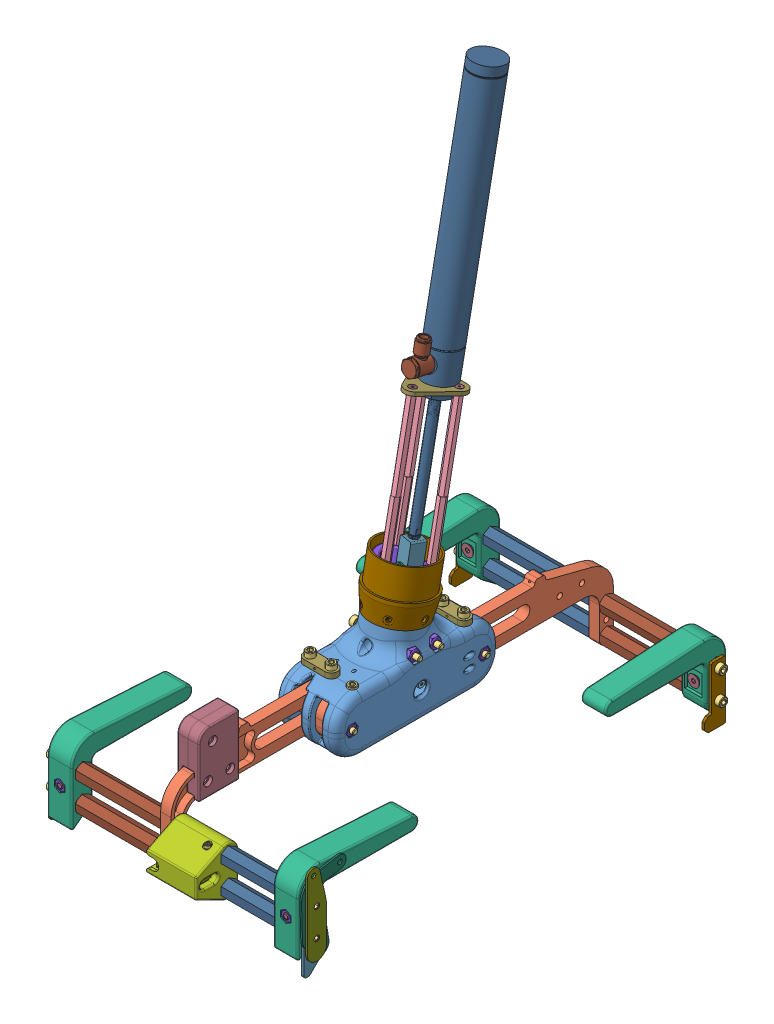
SolidWorks assembly 971-18-A-4000_The Claw, configuration Default. Lengths in mm.
Overall size (243.27 530.53 410.02).
118 component instances, 34 part files, 272 mates.
Components (placement in the parent):
- 971-18-P-0108_Printed Claw Body-1: 971-18-P-0108_Printed Claw Body [Default] at origin size (58.05 92.05 149.22)
- 971-18-P-0077_Main Claw plate-2: 971-18-P-0077_Main Claw plate [Main Claw plate revised] at (9.4298 -158.75 -26.9875) x (0 0 1) z (-1 0 0) size (261.94 82.88 9.53)
- 971-18-P-0077_Main Claw plate-3: 971-18-P-0077_Main Claw plate [Main Claw plate revised] at (-9.4298 -158.75 26.9875) x (0 0 -1) z (1 0 0) size (261.94 82.88 9.53)
- SHCS-1: SHCS [2.25, #10-32] at (3.175 0 -60.325) x (1 0 0) z (0 0.140282 0.990112) size (61.98 7.92 7.92)
- SHCS-2: SHCS [2.25, #10-32] at (3.175 0 60.325) x (1 0 0) z (0 0.980553 -0.196257) size (61.98 7.92 7.92)
- SHCS-3: SHCS [1.875, #10-32] at (-19.177 -1.5875 -50.8) x (0 -1 0) z (-0.074372 0 -0.997231) size (52.45 7.92 7.92)
- SHCS-8: SHCS [2.25, #10-32] at (0 1.5875 -50.8) x (0 -1 0) z (-0.997477 0 -0.07099) size (61.98 7.92 7.92)
- SHCS-9: SHCS [2.25, #10-32] at (19.177 1.5875 -50.8) x (0 -1 0) z (-0.818231 0 -0.57489) size (61.98 7.92 7.92)
- SHCS-10: SHCS [1.875, #10-32] at (19.177 -1.5875 50.8) x (0 -1 0) z (-0.72422 0 -0.689569) size (52.45 7.92 7.92)
- SHCS-11: SHCS [2.25, #10-32] at (0 1.5875 50.8) x (0 -1 0) z (-0.999175 0 0.040609) size (61.98 7.92 7.92)
- SHCS-12: SHCS [2.25, #10-32] at (-19.177 1.5875 50.8) x (0 -1 0) z (0.998979 0 0.045167) size (61.98 7.92 7.92)
- 9433K640_PRECISION STAINLESS STEEL EXTENSION SPRING-1: 9433K640_PRECISION STAINLESS STEEL EXTENSION SPRING [9433K64] at (18.9548 0 -18.9695) x (0 0 1) z (-1 0 0) size (39.67 9.89 9.66)
- 91259A155_ALLOY STEEL SHOULDER SCREW-1: 91259A155_ALLOY STEEL SHOULDER SCREW [91259A155] at (20.5423 0 -7.9375) x (0 -0.354679 -0.934988) z (0 -0.934988 0.354679) size (6.35 13.86 6.35)
- 91259A155_ALLOY STEEL SHOULDER SCREW-2: 91259A155_ALLOY STEEL SHOULDER SCREW [91259A155] at (-20.5423 0 -34.9538) x (0 -0.751431 0.659812) z (0 -0.659812 -0.751431) size (6.35 13.86 6.35)
- 9433K640_PRECISION STAINLESS STEEL EXTENSION SPRING-2: 9433K640_PRECISION STAINLESS STEEL EXTENSION SPRING [9433K64] at (-18.9548 0 20.6375) x (0 0 1) z (-1 0 0) size (39.67 9.89 9.66)
- Bearings-1: Bearings [0.1875 ID, 0.375 OD, 0.125 Width, R166-2Z] at (9.3662 27.94 -18.3873) x (0 -0.996654 0.08174) z (1 0 0) size (9.53 9.53 3.17)
- Bearings-2: Bearings [0.1875 ID, 0.375 OD, 0.125 Width, R166-2Z] at (-9.4932 27.94 1.0215) x (0 -0.380852 0.924636) z (1 0 0) size (9.53 9.53 3.17)
- 971-18-P-0120_Printed Claw Pulley-3: 971-18-P-0120_Printed Claw Pulley [Default] at (-9.4298 27.94 1.0215) x (0 0.87562 0.483001) z (-1 0 0) size (19.05 19.05 4.76)
- 971-18-P-0120_Printed Claw Pulley-4: 971-18-P-0120_Printed Claw Pulley [Default] at (9.4298 27.94 -18.3873) x (0 -0.06152 0.998106) z (-1 0 0) size (19.05 19.05 4.76)
- SHCS-13: SHCS [2.25, #10-32] at (3.175 27.94 -18.3873) x (1 0 0) z (0 0.140282 0.990112) size (61.98 7.92 7.92)
- SHCS-14: SHCS [2.25, #10-32] at (3.175 27.94 1.0215) x (1 0 0) z (0 0.140282 0.990112) size (61.98 7.92 7.92)
- Nylon-Insert Locknut-1: Nylon-Insert Locknut [#10-32 Thin Nylon-Insert Locknut] at (22.225 27.94 1.0215) x (0 -0.5 -0.866025) z (0 -0.866025 0.5) size (9.53 4.37 11)
- Nylon-Insert Locknut-2: Nylon-Insert Locknut [#10-32 Thin Nylon-Insert Locknut] at (22.225 27.94 -18.3873) x (0 1 0) z (0 0 -1) size (9.53 4.37 11)
- Nylon-Insert Locknut-4: Nylon-Insert Locknut [#10-32 Thin Nylon-Insert Locknut] at (24.2094 0 -60.325) x (0 -0.5 -0.866025) z (0 -0.866025 0.5) size (9.53 4.37 11)
- Nylon-Insert Locknut-5: Nylon-Insert Locknut [#10-32 Thin Nylon-Insert Locknut] at (24.2094 0 60.325) x (0 -0.5 0.866025) z (0 0.866025 0.5) size (9.53 4.37 11)
- Nylon-Insert Locknut-14: Nylon-Insert Locknut [#10-32 Thin Nylon-Insert Locknut] at (19.177 -21.0344 50.8) x (0.5 0 0.866025) z (0.866025 0 -0.5) size (9.53 4.37 11)
- Nylon-Insert Locknut-15: Nylon-Insert Locknut [#10-32 Thin Nylon-Insert Locknut] at (0 -21.0344 50.8) x (-0.5 0 -0.866025) z (-0.866025 0 0.5) size (9.53 4.37 11)
- Nylon-Insert Locknut-17: Nylon-Insert Locknut [#10-32 Thin Nylon-Insert Locknut] at (-19.177 -21.0344 50.8) x (-0.5 0 -0.866025) z (-0.866025 0 0.5) size (9.53 4.37 11)
- Nylon-Insert Locknut-18: Nylon-Insert Locknut [#10-32 Thin Nylon-Insert Locknut] at (0 -21.0344 -50.8) x (1 0 0) z (0 0 -1) size (9.53 4.37 11)
- Nylon-Insert Locknut-19: Nylon-Insert Locknut [#10-32 Thin Nylon-Insert Locknut] at (-19.177 -21.0344 -50.8) x (0.5 0 -0.866025) z (-0.866025 0 -0.5) size (9.53 4.37 11)
- Nylon-Insert Locknut-20: Nylon-Insert Locknut [#10-32 Thin Nylon-Insert Locknut] at (19.177 -21.0344 -50.8) x (-0.5 0 0.866025) z (0.866025 0 0.5) size (9.53 4.37 11)
- 971-18-P-0142_Distal Carbon tube adapter-1: 971-18-P-0142_Distal Carbon tube adapter [Default] at (0 89.7497 -17.5007) x (-0.5 -0.165748 -0.850016) z (0 0.981514 -0.19139) size (53.98 53.98 46.99)
- 6498K084_ROUND BODY AIR CYLINDER-1: 6498K084_ROUND BODY AIR CYLINDER [6498K084] at (0 262.1497 -57.0582) x (0 0.981514 -0.19139) z (0 0.19139 0.981514) size (365.16 28.45 28.45)
- 5779K652_PUSH-TO-CONNECT TUBE FITTING FOR AIR-1: 5779K652_PUSH-TO-CONNECT TUBE FITTING FOR AIR [5779K652] at (0 225.7462 -44.6778) x (-1 0 0) z (0 -0.19139 -0.981514) size (14.22 28.59 25.52)
- 971-18-P-0153_Claw Piston Mount-1: 971-18-P-0153_Claw Piston Mount [Default] at (0 207.2186 -46.3469) x (-1 0 0) z (0 -0.19139 -0.981514) size (45.75 3.17 41.53)
- FHCS-15: FHCS [0.25, #4-40] at (-15.7499 209.7238 -50.0883) x (-0.913608 0.077818 0.39908) z (0 0.981514 -0.19139) size (6.48 6.48 6.43)
- FHCS-18: FHCS [0.25, #4-40] at (15.7499 209.7238 -50.0883) x (-0.453098 0.170616 0.874981) z (0 0.981514 -0.19139) size (6.48 6.48 6.43)
- FHCS-17: FHCS [0.25, #4-40] at (0 214.9449 -23.313) x (-0.453098 0.170616 0.874981) z (0 0.981514 -0.19139) size (6.48 6.48 6.43)
- 971-18-P-0162_Claw Piston Cable Block-1: 971-18-P-0162_Claw Piston Cable Block [Default] at (0 80.0327 -21.5464) x (0.973108 0.044086 0.22609) z (-0.230348 0.186243 0.95512) size (12.7 31.75 12.7)
- SHCS-19: SHCS [0.875, #10-32] at (0.7167 71.3508 -22.9383) x (0.230348 -0.186243 -0.95512) z (0.455328 -0.84681 0.274935) size (27.05 7.92 7.92)
- Nylon-Insert Locknut-21: Nylon-Insert Locknut [#10-32 Thin Nylon-Insert Locknut] at (1.843 70.4402 -27.6084) x (-0.550845 -0.834076 0.029792) z (0.802191 -0.51926 0.294719) size (9.53 4.37 11)
- SAE Washer, 18-8 Stainless Steel-1: SAE Washer, 18-8 Stainless Steel [No. 10 Screw SAE Washer] at (-1.6529 73.2667 -13.113) x (0.166548 0.974577 -0.14987) z (0.95875 -0.124551 0.25551) size (12.7 1.65 12.7)
- SAE Washer, 18-8 Stainless Steel-2: SAE Washer, 18-8 Stainless Steel [No. 10 Screw SAE Washer] at (1.6529 70.5939 -26.8199) x (0.166548 0.974577 -0.14987) z (0.95875 -0.124551 0.25551) size (12.7 1.65 12.7)
- FHCS-19: FHCS [0.25, #4-40] at (0 214.9449 -23.313) x (-0.309292 0.182005 0.933388) z (0 0.981514 -0.19139) size (6.48 6.48 6.43)
- Beam Diffuse Sensor-1: Beam Diffuse Sensor [Default] at (2.3678 -35.946 191.135) x (0 -1 0) z (0 0 1) size (12.7 33.5 22.88)
- SHCS-24: SHCS [1, #10-32] at (-103.6637 -29.5056 185.7375) x (1 0 0) z (0 0.235318 -0.971918) size (30.45 7.92 7.92)
- SHCS-26: SHCS [1.5, #4-40] at (30.5617 -43.439 194.183) x (0 -1 0) z (0.977714 0 0.209939) size (40.94 4.65 4.65)
- SHCS-33: SHCS [1, #10-32] at (103.6637 -29.5056 185.7375) x (-1 0 0) z (0 0.845438 -0.534073) size (30.45 7.92 7.92)
- SHCS-35: SHCS [1, #10-32] at (103.6637 -54.9056 185.7375) x (-1 0 0) z (0 -0.631694 -0.775218) size (30.45 7.92 7.92)
- SHCS-37: SHCS [1, #10-32] at (103.6637 -29.5056 -185.7375) x (-1 0 0) z (0 -0.058563 -0.998284) size (30.45 7.92 7.92)
- SHCS-39: SHCS [1, #10-32] at (103.6637 -54.9056 -185.7375) x (-1 0 0) z (0 -0.744643 -0.667463) size (30.45 7.92 7.92)
- SHCS-41: SHCS [1, #10-32] at (-103.6637 -54.9056 -185.7375) x (1 0 0) z (0 0.359883 -0.932997) size (30.45 7.92 7.92)
- SHCS-43: SHCS [1, #10-32] at (-103.6637 -29.5056 -185.7375) x (1 0 0) z (0 0.980192 0.198051) size (30.45 7.92 7.92)
- 92311A433_18-8 SS CUP POINT SET SCREW-1: 92311A433_18-8 SS CUP POINT SET SCREW [92311A433] at (-10.0105 -54.9056 185.7375) x (0 -0.712759 -0.701409) z (-1 0 0) size (4.99 4.84 25.82)
- 92311A433_18-8 SS CUP POINT SET SCREW-5: 92311A433_18-8 SS CUP POINT SET SCREW [92311A433] at (-11.02 -29.5056 185.7375) x (0 -0.999929 0.011906) z (1 0 0) size (4.99 4.84 25.82)
- 93365A142_BRASS HEAT-SET INSERT FOR PLASTICS-1: 93365A142_BRASS HEAT-SET INSERT FOR PLASTICS [93365A142] at (-11.1125 53.5447 9.169) x (0.785545 0.5 0.36458) z (0.36458 -0.850016 0.380203) size (6.35 8.46 6.35)
- 93365A142_BRASS HEAT-SET INSERT FOR PLASTICS-2: 93365A142_BRASS HEAT-SET INSERT FOR PLASTICS [93365A142] at (-22.225 49.8609 -9.7226) x (0 0.545272 0.838259) z (0 -0.838259 0.545272) size (6.35 8.46 6.35)
- 93365A142_BRASS HEAT-SET INSERT FOR PLASTICS-4: 93365A142_BRASS HEAT-SET INSERT FOR PLASTICS [93365A142] at (-11.1125 46.1772 -28.6142) x (-0.813186 -0.24774 0.526644) z (0.297873 -0.954543 0.010914) size (6.35 8.46 6.35)
- 93365A142_BRASS HEAT-SET INSERT FOR PLASTICS-6: 93365A142_BRASS HEAT-SET INSERT FOR PLASTICS [93365A142] at (11.1125 46.1772 -28.6142) x (0.371763 0.927557 0.037811) z (-0.782172 0.33491 -0.525398) size (6.35 8.46 6.35)
- 93365A142_BRASS HEAT-SET INSERT FOR PLASTICS-8: 93365A142_BRASS HEAT-SET INSERT FOR PLASTICS [93365A142] at (22.225 49.8609 -9.7226) x (0 0.873561 -0.486714) z (0 -0.486714 -0.873561) size (6.35 8.46 6.35)
- 93365A142_BRASS HEAT-SET INSERT FOR PLASTICS-10: 93365A142_BRASS HEAT-SET INSERT FOR PLASTICS [93365A142] at (11.1125 53.5447 9.169) x (0.459987 0.780789 -0.422825) z (0.733766 -0.602409 -0.314152) size (6.35 8.46 6.35)
- 92311A433_18-8 SS CUP POINT SET SCREW-11: 92311A433_18-8 SS CUP POINT SET SCREW [92311A433] at (9.2914 -29.5056 -185.7375) x (0 0.990314 -0.138846) z (1 0 0) size (4.99 4.84 25.82)
- 92311A433_18-8 SS CUP POINT SET SCREW-14: 92311A433_18-8 SS CUP POINT SET SCREW [92311A433] at (9.9158 -54.9056 -185.7375) x (0 -0.994426 -0.105437) z (1 0 0) size (4.99 4.84 25.82)
- 94638A222_NYLON UNTHREADED SPACERS-1: 94638A222_NYLON UNTHREADED SPACERS [94638A222] at (-19.177 0 50.8) x (1 0 0) z (0 1 0) size (9.53 9.53 33.34)
- 94638A222_NYLON UNTHREADED SPACERS-2: 94638A222_NYLON UNTHREADED SPACERS [94638A222] at (-19.177 0 -50.8) x (1 0 0) z (0 1 0) size (9.53 9.53 33.34)
- 94638A222_NYLON UNTHREADED SPACERS-3: 94638A222_NYLON UNTHREADED SPACERS [94638A222] at (19.177 0 -50.8) x (1 0 0) z (0 1 0) size (9.53 9.53 33.34)
- 94639A550_NYLON UNTHREADED SPACERS-1: 94639A550_NYLON UNTHREADED SPACERS [94639A550] at (-9.4298 0 -60.325) x (0 -0.918334 -0.395806) z (1 0 0) size (12.7 12.7 9.53)
- 94639A586_NYLON UNTHREADED SPACERS-1: 94639A586_NYLON UNTHREADED SPACERS [94639A586] at (0 11.9062 50.8) x (1 0 0) z (0 1 0) size (9.53 9.53 10.32)
- 94638A222_NYLON UNTHREADED SPACERS-4: 94638A222_NYLON UNTHREADED SPACERS [94638A222] at (19.177 0 50.8) x (1 0 0) z (0 1 0) size (9.53 9.53 33.34)
- 94639A550_NYLON UNTHREADED SPACERS-2: 94639A550_NYLON UNTHREADED SPACERS [94639A550] at (9.4298 0 -60.325) x (0 -0.323653 0.946176) z (-1 0 0) size (12.7 12.7 9.53)
- 94639A550_NYLON UNTHREADED SPACERS-3: 94639A550_NYLON UNTHREADED SPACERS [94639A550] at (-9.4298 0 60.325) x (0 -0.362888 0.931833) z (-1 0 0) size (12.7 12.7 9.53)
- 94639A550_NYLON UNTHREADED SPACERS-4: 94639A550_NYLON UNTHREADED SPACERS [94639A550] at (9.4298 0 60.325) x (0 -0.966697 0.255924) z (-1 0 0) size (12.7 12.7 9.53)
- 94639A586_NYLON UNTHREADED SPACERS-2: 94639A586_NYLON UNTHREADED SPACERS [94639A586] at (0 11.9062 -50.8) x (1 0 0) z (0 1 0) size (9.53 9.53 10.32)
- 94639A586_NYLON UNTHREADED SPACERS-3: 94639A586_NYLON UNTHREADED SPACERS [94639A586] at (0 -11.9062 50.8) x (1 0 0) z (0 1 0) size (9.53 9.53 10.32)
- 94639A586_NYLON UNTHREADED SPACERS-4: 94639A586_NYLON UNTHREADED SPACERS [94639A586] at (0 -11.9062 -50.8) x (1 0 0) z (0 1 0) size (9.53 9.53 10.32)
- 91780A049_ALUM FEM THRDED HEX STANDOFF-1: 91780A049_ALUM FEM THRDED HEX STANDOFF [91780A049] at (0 174.4329 -15.4133) x (0.203683 0.187378 0.960938) z (0 -0.981514 0.19139) size (6.35 7.33 76.64)
- 98637A123_ALLOY STEEL MIL SPEC CUP POINT SET SCREW-1: 98637A123_ALLOY STEEL MIL SPEC CUP POINT SET SCREW [98637A123] at (0 134.5273 -7.632) x (0.994254 0.020488 0.105072) z (0 -0.981514 0.19139) size (3.28 2.93 13.1)
- SHCS-44: SHCS [1, #10-32] at (-103.6637 -54.9056 185.7375) x (1 0 0) z (0 0.985655 0.168775) size (30.45 7.92 7.92)
- 91780A049_ALUM FEM THRDED HEX STANDOFF-2: 91780A049_ALUM FEM THRDED HEX STANDOFF [91780A049] at (15.7499 94.4205 -27.6048) x (-0.911227 0.078834 0.404291) z (0 0.981514 -0.19139) size (6.35 7.33 76.64)
- 91780A049_ALUM FEM THRDED HEX STANDOFF-3: 91780A049_ALUM FEM THRDED HEX STANDOFF [91780A049] at (-15.7499 169.2118 -42.1887) x (1 0 0) z (0 0.981514 -0.19139) size (6.35 7.33 76.64)
- 91780A049_ALUM FEM THRDED HEX STANDOFF-4: 91780A049_ALUM FEM THRDED HEX STANDOFF [91780A049] at (-15.7499 94.4205 -27.6048) x (-0.005423 -0.191387 -0.9815) z (0 -0.981514 0.19139) size (6.35 7.33 76.64)
- 91780A049_ALUM FEM THRDED HEX STANDOFF-5: 91780A049_ALUM FEM THRDED HEX STANDOFF [91780A049] at (15.7499 169.2118 -42.1887) x (-0.577436 0.156258 0.801344) z (0 0.981514 -0.19139) size (6.35 7.33 76.64)
- 91780A049_ALUM FEM THRDED HEX STANDOFF-6: 91780A049_ALUM FEM THRDED HEX STANDOFF [91780A049] at (0 99.6415 -0.8294) x (0.866025 -0.095695 -0.490757) z (0 -0.981514 0.19139) size (6.35 7.33 76.64)
- 98637A123_ALLOY STEEL MIL SPEC CUP POINT SET SCREW-2: 98637A123_ALLOY STEEL MIL SPEC CUP POINT SET SCREW [98637A123] at (-15.7499 132.8293 -35.0943) x (-0.962053 0.052223 0.267819) z (0 0.981514 -0.19139) size (3.28 2.93 13.1)
- 98637A123_ALLOY STEEL MIL SPEC CUP POINT SET SCREW-3: 98637A123_ALLOY STEEL MIL SPEC CUP POINT SET SCREW [98637A123] at (15.7499 131.8727 -34.9077) x (-0.341225 -0.179903 -0.922605) z (0 -0.981514 0.19139) size (3.28 2.93 13.1)
- 971-18-P-0299_Printed Claw Ends-1: 971-18-P-0299_Printed Claw Ends [Default] at (102.9652 -29.5056 -185.7375) size (22.23 68.03 110.13)
- 971-18-P-0299_Printed Claw Ends-2: 971-18-P-0299_Printed Claw Ends [Default] at (-102.9652 -29.5056 -185.7375) size (22.23 68.03 110.13)
- 971-18-P-0299_Printed Claw Ends-3: 971-18-P-0299_Printed Claw Ends [Default] at (-102.9652 -29.5056 185.7375) x (-1 0 0) z (0 0 -1) size (22.23 68.03 110.13)
- 971-18-P-0299_Printed Claw Ends-4: 971-18-P-0299_Printed Claw Ends [Default] at (102.9652 -29.5056 185.7375) x (-1 0 0) z (0 0 -1) size (22.23 68.03 110.13)
- 971-18-P-0300_Printed Claw Beam Break Mount-1: 971-18-P-0300_Printed Claw Beam Break Mount [Default] at (18.1928 -29.469 185.801) x (-1 0 0) z (0 0 -1) size (45.72 44.45 38.48)
- Nylon-Insert Locknut-22: Nylon-Insert Locknut [#10-32 Thin Nylon-Insert Locknut] at (102.9652 -42.2056 190.5) x (-0.998457 -0.055527 0) z (-0.055527 0.998457 0) size (9.53 4.37 11)
- FHCS-20: FHCS [0.75, #10-32] at (102.9652 -42.2056 176.2125) x (-0.923728 -0.383049 0) z (0 0 -1) size (10.44 10.44 19.21)
- FHCS-21: FHCS [0.75, #10-32] at (-102.9652 -42.2056 176.2125) x (-0.873774 -0.486332 0) z (0 0 -1) size (10.44 10.44 19.21)
- FHCS-24: FHCS [0.75, #10-32] at (-102.9652 -42.2056 -176.2125) x (-0.044015 -0.999031 0) z (0 0 1) size (10.44 10.44 19.21)
- FHCS-26: FHCS [0.75, #10-32] at (102.9652 -42.2056 -176.2125) x (0.130134 -0.991496 0) z (0 0 1) size (10.44 10.44 19.21)
- Nylon-Insert Locknut-23: Nylon-Insert Locknut [#10-32 Thin Nylon-Insert Locknut] at (-102.9652 -42.2056 190.5) x (-0.985526 -0.169524 0) z (-0.169524 0.985526 0) size (9.53 4.37 11)
- Nylon-Insert Locknut-25: Nylon-Insert Locknut [#10-32 Thin Nylon-Insert Locknut] at (-102.9652 -42.2056 -190.5) x (0.289314 -0.957234 0) z (0.957234 0.289314 0) size (9.53 4.37 11)
- Nylon-Insert Locknut-27: Nylon-Insert Locknut [#10-32 Thin Nylon-Insert Locknut] at (102.9652 -42.2056 -190.5) x (0.451141 -0.892453 0) z (0.892453 0.451141 0) size (9.53 4.37 11)
- 971-18-P-0304_Claw Standoff Ring-1: 971-18-P-0304_Claw Standoff Ring [Default] at (0 65.555 -12.7829) x (0.5 0.165748 0.850016) z (-0.866025 0.095695 0.490757) size (43.02 19.34 44.45)
- 971-18-P-0312_Claw Fangs-1: 971-18-P-0312_Claw Fangs [Default] at (114.0778 -76.4956 200.7755) size (2.29 53.34 19.05) (hidden)
- 971-18-P-0312_Claw Fangs-6: 971-18-P-0312_Claw Fangs [Default] at (-114.0778 -76.4956 -200.7755) x (-1 0 0) z (0 0 -1) size (2.29 53.34 19.05)
- 971-18-P-0312_Claw Fangs-11: 971-18-P-0312_Claw Fangs [Default] at (116.3637 -76.4956 -200.7755) x (-1 0 0) z (0 0 -1) size (2.29 53.34 19.05)
- 971-18-P-0312_Claw Fangs-12: 971-18-P-0312_Claw Fangs [Default] at (-116.3637 -76.4956 200.7755) size (2.29 53.34 19.05)
- 971-18-P-0316_Claw Long Horizontal Standoff-1: 971-18-P-0316_Claw Long Horizontal Standoff [91780A354] at (-46.1328 -54.9056 -185.7375) x (0 0.866025 -0.5) z (1 0 0) size (12.7 14.66 102.22)
- 971-18-P-0317_Claw Short Horizontal Standoff-1: 971-18-P-0317_Claw Short Horizontal Standoff [91780A354] at (-91.8528 -54.9056 185.7375) x (0 -0.912023 0.41014) z (1 0 0) size (12.7 14.66 82.74)
- 971-18-P-0317_Claw Short Horizontal Standoff-2: 971-18-P-0317_Claw Short Horizontal Standoff [91780A354] at (91.8528 -54.9056 -185.7375) x (0 -0.866025 0.5) z (-1 0 0) size (12.7 14.66 82.74)
- 971-18-P-0317_Claw Short Horizontal Standoff-3: 971-18-P-0317_Claw Short Horizontal Standoff [91780A354] at (91.8528 -29.5056 -185.7375) x (0 0.196892 -0.980425) z (-1 0 0) size (12.7 14.66 82.74)
- 971-18-P-0317_Claw Short Horizontal Standoff-4: 971-18-P-0317_Claw Short Horizontal Standoff [91780A354] at (-91.8528 -29.5056 185.7375) x (0 0.866025 -0.5) z (1 0 0) size (12.7 14.66 82.74)
- 971-18-P-0316_Claw Long Horizontal Standoff-2: 971-18-P-0316_Claw Long Horizontal Standoff [91780A354] at (46.1328 -29.5056 185.7375) x (0 0 1) z (-1 0 0) size (12.7 14.66 102.22)
- 971-18-P-0316_Claw Long Horizontal Standoff-3: 971-18-P-0316_Claw Long Horizontal Standoff [91780A354] at (-46.1328 -29.5056 -185.7375) x (0 0.866025 -0.5) z (1 0 0) size (12.7 14.66 102.22)
- 971-18-P-0316_Claw Long Horizontal Standoff-4: 971-18-P-0316_Claw Long Horizontal Standoff [91780A354] at (46.1328 -54.9056 185.7375) x (0 0.866025 -0.5) z (-1 0 0) size (12.7 14.66 102.22)
- 971-18-P-0326_Claw Cable Holder-2: 971-18-P-0326_Claw Cable Holder [Default] at (-19.177 30.1625 50.8) x (1 0 0) z (0 0 -1) size (30.61 4.76 11.43)
- 971-18-P-0326_Claw Cable Holder-3: 971-18-P-0326_Claw Cable Holder [Default] at (0 30.1625 -50.8) x (1 0 0) z (0 0 -1) size (30.61 4.76 11.43)
- 971-18-P-0318_Claw Pulley Mount-5: 971-18-P-0318_Claw Pulley Mount [971-18-P-0318_Claw Pulley Mount] at (-19.2722 5.212 171.7608) x (0 0 -1) z (1 0 0) size (36.91 55.31 10.39)
- 971-18-P-0318_Claw Pulley Mount-6: 971-18-P-0318_Claw Pulley Mount [971-18-P-0330_Claw Pulley Mount Inner Side] at (-9.4298 5.212 171.7608) x (0 0 -1) z (1 0 0) size (36.91 55.31 11.43)
- 971-18-P-0361_Claw Fangs V2-1: 971-18-P-0361_Claw Fangs V2 [Default] at (115.2207 -29.5056 185.7375) size (2.29 63.5 20.32)
- 971-18-P-0367_Retrofit Fang Sheath-1: 971-18-P-0367_Retrofit Fang Sheath [Default] at (116.3637 -29.5056 185.7375) x (1 0 0) z (0 -0.027695 0.999616) size (1.52 70.53 41.08)
- 971-18-P-0368_Retrofit Fang Sheath Outside-1: 971-18-P-0368_Retrofit Fang Sheath Outside [Default] at (120.3325 -29.5056 185.7375) size (1.52 74.51 17.53)
Mates (geometry in assembly coordinates):
- Coincident5: coincident aligned: plane of 971-18-P-0108_Printed Claw Body-1 through (0 0 0) normal (0 0 1); plane of assembly through (0 0 0) normal (0 0 1)
- Coincident6: coincident aligned: plane of 971-18-P-0108_Printed Claw Body-1 through (0 0 0) normal (0 1 0); plane of assembly through (0 0 0) normal (0 1 0)
- Coincident7: coincident aligned: plane of 971-18-P-0108_Printed Claw Body-1 through (0 0 0) normal (1 0 0); plane of assembly through (0 0 0) normal (1 0 0)
- Width1: width anti-aligned: plane of 971-18-P-0108_Printed Claw Body-1 through (15.0495 17.4625 -74.6125) normal (-1 0 0); plane of 971-18-P-0077_Main Claw plate-2 through (3.81 17.4625 -74.6125) normal (1 0 0); plane of 971-18-P-0108_Printed Claw Body-1 through (14.1922 -158.75 -26.9875) normal (1 0 0); plane of 971-18-P-0077_Main Claw plate-2 through (4.6673 -158.75 -26.9875) normal (-1 0 0)
- Width3: width anti-aligned: plane of 971-18-P-0108_Printed Claw Body-1 through (-15.0495 17.4625 -74.6125) normal (1 0 0); plane of 971-18-P-0077_Main Claw plate-3 through (-3.81 17.4625 -74.6125) normal (-1 0 0); plane of 971-18-P-0108_Printed Claw Body-1 through (-14.1922 -158.75 26.9875) normal (-1 0 0); plane of 971-18-P-0077_Main Claw plate-3 through (-4.6673 -158.75 26.9875) normal (1 0 0)
- Symmetric3: symmetric aligned: plane of 971-18-P-0077_Main Claw plate-2 through (4.6673 -15.875 69.85) normal (0 0 1); plane of 971-18-P-0077_Main Claw plate-3 through (-4.6673 -15.875 -69.85) normal (0 0 -1); plane of assembly through (0 0 0) normal (0 0 1)
- Concentric10: concentric anti-aligned: cylinder of 971-18-P-0108_Printed Claw Body-1 through (28.575 0 -60.325) axis (-1 0 0) radius 2.5527; cylinder of SHCS-1 through (-25.4 0 -60.325) axis (1 0 0) radius 2.413
- Concentric12: concentric anti-aligned: cylinder of 971-18-P-0108_Printed Claw Body-1 through (28.575 0 60.325) axis (-1 0 0) radius 2.5527; cylinder of SHCS-2 through (-25.4 0 60.325) axis (1 0 0) radius 2.413
- Concentric13: concentric anti-aligned: cylinder of 971-18-P-0108_Printed Claw Body-1 through (-19.177 25.4 -50.8) axis (0 1 0) radius 2.4574; cylinder of SHCS-3 through (-19.177 22.225 -50.8) axis (0 -1 0) radius 2.413
- Concentric18: concentric anti-aligned: cylinder of 971-18-P-0108_Printed Claw Body-1 through (0 25.4 -50.8) axis (0 1 0) radius 2.4574; cylinder of SHCS-8 through (0 30.1625 -50.8) axis (0 -1 0) radius 2.413
- Concentric19: concentric anti-aligned: cylinder of 971-18-P-0108_Printed Claw Body-1 through (19.177 25.4 -50.8) axis (0 1 0) radius 2.4574; cylinder of SHCS-9 through (19.177 30.1625 -50.8) axis (0 -1 0) radius 2.413
- Concentric20: concentric anti-aligned: cylinder of 971-18-P-0108_Printed Claw Body-1 through (19.177 25.4 50.8) axis (0 1 0) radius 2.4574; cylinder of SHCS-10 through (19.177 22.225 50.8) axis (0 -1 0) radius 2.413
- Concentric21: concentric anti-aligned: cylinder of 971-18-P-0108_Printed Claw Body-1 through (0 25.4 50.8) axis (0 1 0) radius 2.4574; cylinder of SHCS-11 through (0 30.1625 50.8) axis (0 -1 0) radius 2.413
- Concentric22: concentric anti-aligned: cylinder of 971-18-P-0108_Printed Claw Body-1 through (-19.177 25.4 50.8) axis (0 1 0) radius 2.4574; cylinder of SHCS-12 through (-19.177 30.1625 50.8) axis (0 -1 0) radius 2.413
- Coincident23: coincident aligned: plane of 9433K640_PRECISION STAINLESS STEEL EXTENSION SPRING-1 through (18.9548 0 -18.9695) normal (0 1 0); plane of assembly through (0 0 0) normal (0 1 0)
- Distance3: distance = 4.7625 mm anti-aligned: plane of 9433K640_PRECISION STAINLESS STEEL EXTENSION SPRING-1 through (18.9548 0 -18.9695) normal (-1 0 0); plane of 971-18-P-0077_Main Claw plate-2 through (14.1922 -158.75 -26.9875) normal (1 0 0)
- Concentric28: concentric aligned: cylinder of 971-18-P-0077_Main Claw plate-2 through (4.6673 0 -7.9375) axis (-1 0 0) radius 1.1303; cylinder of 91259A155_ALLOY STEEL SHOULDER SCREW-1 through (20.5423 0 -7.9375) axis (-1 0 0) radius 1.5875
- Coincident25: coincident anti-aligned: plane of 971-18-P-0077_Main Claw plate-2 through (14.1922 -158.75 -26.9875) normal (1 0 0); plane of 91259A155_ALLOY STEEL SHOULDER SCREW-1 through (14.1922 0 -7.9375) normal (-1 0 0)
- Coincident26: coincident anti-aligned: plane of 971-18-P-0077_Main Claw plate-3 through (-14.1922 -158.75 26.9875) normal (-1 0 0); plane of 91259A155_ALLOY STEEL SHOULDER SCREW-2 through (-14.1922 0 -34.9538) normal (1 0 0)
- Coincident27: coincident aligned: plane of 9433K640_PRECISION STAINLESS STEEL EXTENSION SPRING-2 through (-18.9548 0 20.6375) normal (0 1 0); plane of assembly through (0 0 0) normal (0 1 0)
- Distance4: distance = 4.7625 mm aligned: plane of 9433K640_PRECISION STAINLESS STEEL EXTENSION SPRING-2 through (-18.9548 0 20.6375) normal (-1 0 0); plane of 971-18-P-0077_Main Claw plate-3 through (-14.1922 -158.75 26.9875) normal (-1 0 0)
- Concentric32: concentric anti-aligned: cylinder of 971-18-P-0108_Printed Claw Body-1 through (30.2619 27.94 1.0215) axis (-1 0 0) radius 2.3813; cylinder of Bearings-2 through (-3.6127 27.94 1.0215) axis (1 0 0) radius 2.3813
- Concentric33: concentric anti-aligned: cylinder of 971-18-P-0108_Printed Claw Body-1 through (30.2619 27.94 -18.3873) axis (-1 0 0) radius 2.3813; cylinder of Bearings-1 through (15.2468 27.94 -18.3873) axis (1 0 0) radius 2.3813
- Width19: width anti-aligned: plane of 971-18-P-0108_Printed Claw Body-1 through (12.6047 27.94 -18.3873) normal (-1 0 0); plane of 971-18-P-0120_Printed Claw Pulley-4 through (6.2547 27.94 -18.3873) normal (1 0 0); plane of 971-18-P-0108_Printed Claw Body-1 through (11.811 37.447 -17.8014) normal (1 0 0); plane of 971-18-P-0120_Printed Claw Pulley-4 through (7.0485 37.447 -17.8014) normal (-1 0 0)
- Width20: width anti-aligned: plane of 971-18-P-0108_Printed Claw Body-1 through (-6.2547 27.94 1.0215) normal (-1 0 0); plane of 971-18-P-0120_Printed Claw Pulley-3 through (-12.6047 27.94 1.0215) normal (1 0 0); plane of 971-18-P-0108_Printed Claw Body-1 through (-7.0485 32.5406 -7.3188) normal (1 0 0); plane of 971-18-P-0120_Printed Claw Pulley-3 through (-11.811 32.5406 -7.3188) normal (-1 0 0)
- Coincident30: coincident anti-aligned: plane of 971-18-P-0108_Printed Claw Body-1 through (-25.4 0 60.325) normal (-1 0 0); plane of SHCS-2 through (-25.4 -0.7303 56.6763) normal (1 0 0)
- Coincident31: coincident anti-aligned: plane of 971-18-P-0108_Printed Claw Body-1 through (-25.4 0 -60.325) normal (-1 0 0); plane of SHCS-1 through (-25.4 3.6843 -60.847) normal (1 0 0)
- Coincident32: coincident anti-aligned: plane of 971-18-P-0108_Printed Claw Body-1 through (19.177 22.225 50.8) normal (0 1 0); plane of SHCS-10 through (16.611 22.225 53.4949) normal (0 -1 0)
- Coincident38: coincident anti-aligned: plane of 971-18-P-0108_Printed Claw Body-1 through (-19.177 22.225 -50.8) normal (0 1 0); plane of SHCS-3 through (-22.8878 22.225 -50.5233) normal (0 -1 0)
- Concentric36: concentric anti-aligned: cylinder of 971-18-P-0108_Printed Claw Body-1 through (30.2619 27.94 1.0215) axis (-1 0 0) radius 2.3813; cylinder of SHCS-14 through (-25.4 27.94 1.0215) axis (1 0 0) radius 2.413
- Concentric37: concentric anti-aligned: cylinder of 971-18-P-0108_Printed Claw Body-1 through (30.2619 27.94 -18.3873) axis (-1 0 0) radius 2.3813; cylinder of SHCS-13 through (-25.4 27.94 -18.3873) axis (1 0 0) radius 2.413
- Coincident39: coincident anti-aligned: plane of 971-18-P-0108_Printed Claw Body-1 through (-25.4 27.94 -18.3873) normal (-1 0 0); plane of SHCS-13 through (-25.4 31.6243 -18.9093) normal (1 0 0)
- Coincident40: coincident anti-aligned: plane of 971-18-P-0108_Printed Claw Body-1 through (-25.4 27.94 1.0215) normal (-1 0 0); plane of SHCS-14 through (-25.4 31.6243 0.4994) normal (1 0 0)
- Concentric38: concentric anti-aligned: cylinder of SHCS-14 through (-25.4 27.94 1.0215) axis (1 0 0) radius 2.413; cylinder of Nylon-Insert Locknut-1 through (19.812 27.94 1.0215) axis (-1 0 0) radius 2.413
- Coincident41: coincident anti-aligned: plane of 971-18-P-0108_Printed Claw Body-1 through (22.225 0 0) normal (1 0 0); plane of Nylon-Insert Locknut-1 through (22.225 32.7025 -1.7282) normal (-1 0 0)
- Parallel1: parallel aligned: plane of 971-18-P-0108_Printed Claw Body-1 through (22.225 23.1775 3.7711) normal (0 1 0); plane of Nylon-Insert Locknut-1 through (26.5906 32.7025 -1.7282) normal (0 1 0)
- Concentric39: concentric anti-aligned: cylinder of SHCS-13 through (-25.4 27.94 -18.3873) axis (1 0 0) radius 2.413; cylinder of Nylon-Insert Locknut-2 through (19.812 27.94 -18.3873) axis (-1 0 0) radius 2.413
- Parallel2: parallel aligned: plane of 971-18-P-0108_Printed Claw Body-1 through (22.225 23.1775 -15.6377) normal (0 1 0); plane of Nylon-Insert Locknut-2 through (26.5906 32.7025 -21.137) normal (0 1 0)
- Coincident44: coincident anti-aligned: plane of 971-18-P-0108_Printed Claw Body-1 through (22.225 0 0) normal (1 0 0); plane of Nylon-Insert Locknut-2 through (22.225 27.94 -12.8881) normal (-1 0 0)
- Concentric40: concentric anti-aligned: cylinder of SHCS-1 through (-25.4 0 -60.325) axis (1 0 0) radius 2.413; cylinder of Nylon-Insert Locknut-4 through (21.7964 0 -60.325) axis (-1 0 0) radius 2.413
- Coincident47: coincident anti-aligned: plane of 971-18-P-0108_Printed Claw Body-1 through (24.2094 0 0) normal (1 0 0); plane of Nylon-Insert Locknut-4 through (24.2094 4.7625 -63.0746) normal (-1 0 0)
- Parallel3: parallel aligned: plane of Nylon-Insert Locknut-4 through (28.575 -4.7625 -57.5754) normal (0 -1 0); plane of 971-18-P-0108_Printed Claw Body-1 through (24.2094 4.7625 -63.0746) normal (0 -1 0)
- Concentric41: concentric anti-aligned: cylinder of SHCS-2 through (-25.4 0 60.325) axis (1 0 0) radius 2.413; cylinder of Nylon-Insert Locknut-5 through (21.7964 0 60.325) axis (-1 0 0) radius 2.413
- Coincident50: coincident anti-aligned: plane of 971-18-P-0108_Printed Claw Body-1 through (24.2094 0 65.8243) normal (0 0.5 -0.866025); plane of Nylon-Insert Locknut-5 through (28.575 0 65.8243) normal (0 -0.5 0.866025)
- Coincident51: coincident anti-aligned: plane of 971-18-P-0108_Printed Claw Body-1 through (24.2094 0 0) normal (1 0 0); plane of Nylon-Insert Locknut-5 through (24.2094 -4.7625 57.5754) normal (-1 0 0)
- Concentric45: concentric anti-aligned: cylinder of SHCS-10 through (19.177 22.225 50.8) axis (0 -1 0) radius 2.413; cylinder of Nylon-Insert Locknut-14 through (19.177 -18.6214 50.8) axis (0 1 0) radius 2.413
- Coincident59: coincident anti-aligned: plane of 971-18-P-0108_Printed Claw Body-1 through (19.177 -21.0344 45.3007) normal (-0.5 0 0.866025); plane of Nylon-Insert Locknut-14 through (19.177 -25.4 45.3007) normal (0.5 0 -0.866025)
- Coincident60: coincident anti-aligned: plane of 971-18-P-0108_Printed Claw Body-1 through (0 -21.0344 0) normal (0 -1 0); plane of Nylon-Insert Locknut-14 through (14.4145 -21.0344 53.5496) normal (0 1 0)
- Concentric47: concentric anti-aligned: cylinder of SHCS-11 through (0 30.1625 50.8) axis (0 -1 0) radius 2.413; cylinder of Nylon-Insert Locknut-15 through (0 -18.6214 50.8) axis (0 1 0) radius 2.413
- Coincident63: coincident anti-aligned: plane of 971-18-P-0108_Printed Claw Body-1 through (0 -21.0344 45.3007) normal (-0.5 0 0.866025); plane of Nylon-Insert Locknut-15 through (0 -25.4 45.3007) normal (0.5 0 -0.866025)
- Coincident64: coincident anti-aligned: plane of 971-18-P-0108_Printed Claw Body-1 through (0 -21.0344 0) normal (0 -1 0); plane of Nylon-Insert Locknut-15 through (4.7625 -21.0344 48.0504) normal (0 1 0)
- Concentric49: concentric anti-aligned: cylinder of SHCS-12 through (-19.177 30.1625 50.8) axis (0 -1 0) radius 2.413; cylinder of Nylon-Insert Locknut-17 through (-19.177 -18.6214 50.8) axis (0 1 0) radius 2.413
- Coincident65: coincident anti-aligned: plane of 971-18-P-0108_Printed Claw Body-1 through (-19.177 -21.0344 45.3007) normal (-0.5 0 0.866025); plane of Nylon-Insert Locknut-17 through (-19.177 -25.4 45.3007) normal (0.5 0 -0.866025)
- Coincident66: coincident anti-aligned: plane of 971-18-P-0108_Printed Claw Body-1 through (0 -21.0344 0) normal (0 -1 0); plane of Nylon-Insert Locknut-17 through (-14.4145 -21.0344 48.0504) normal (0 1 0)
- Concentric50: concentric anti-aligned: cylinder of SHCS-9 through (19.177 30.1625 -50.8) axis (0 -1 0) radius 2.413; cylinder of Nylon-Insert Locknut-20 through (19.177 -18.6214 -50.8) axis (0 1 0) radius 2.413
- Coincident68: coincident anti-aligned: plane of 971-18-P-0108_Printed Claw Body-1 through (23.9395 -21.0344 -53.5496) normal (-1 0 0); plane of Nylon-Insert Locknut-20 through (23.9395 -25.4 -53.5496) normal (1 0 0)
- Coincident70: coincident anti-aligned: plane of 971-18-P-0108_Printed Claw Body-1 through (0 -21.0344 0) normal (0 -1 0); plane of Nylon-Insert Locknut-20 through (14.4145 -21.0344 -53.5496) normal (0 1 0)
- Concentric52: concentric anti-aligned: cylinder of SHCS-8 through (0 30.1625 -50.8) axis (0 -1 0) radius 2.413; cylinder of Nylon-Insert Locknut-18 through (0 -18.6214 -50.8) axis (0 1 0) radius 2.413
- Coincident71: coincident anti-aligned: plane of 971-18-P-0108_Printed Claw Body-1 through (-4.7625 -21.0344 -53.5496) normal (0.5 0 0.866025); plane of Nylon-Insert Locknut-18 through (-4.7625 -25.4 -53.5496) normal (-0.5 0 -0.866025)
- Coincident72: coincident anti-aligned: plane of 971-18-P-0108_Printed Claw Body-1 through (0 -21.0344 0) normal (0 -1 0); plane of Nylon-Insert Locknut-18 through (0 -21.0344 -45.3007) normal (0 1 0)
- Concentric53: concentric anti-aligned: cylinder of SHCS-3 through (-19.177 22.225 -50.8) axis (0 -1 0) radius 2.413; cylinder of Nylon-Insert Locknut-19 through (-19.177 -18.6214 -50.8) axis (0 1 0) radius 2.413
- Coincident73: coincident anti-aligned: plane of 971-18-P-0108_Printed Claw Body-1 through (-23.9395 -21.0344 -53.5496) normal (0.5 0 0.866025); plane of Nylon-Insert Locknut-19 through (-23.9395 -25.4 -53.5496) normal (-0.5 0 -0.866025)
- Coincident74: coincident anti-aligned: plane of 971-18-P-0108_Printed Claw Body-1 through (0 -21.0344 0) normal (0 -1 0); plane of Nylon-Insert Locknut-19 through (-14.4145 -21.0344 -48.0504) normal (0 1 0)
- Concentric54: concentric aligned: cylinder of 971-18-P-0108_Printed Claw Body-1 through (0 43.6283 -8.5073) axis (0 0.981514 -0.19139) radius 22.225; cylinder of 971-18-P-0142_Distal Carbon tube adapter-1 through (0 89.7497 -17.5007) axis (0 0.981514 -0.19139) radius 22.225
- Coincident75: coincident anti-aligned: plane of 971-18-P-0108_Printed Claw Body-1 through (0 44.3804 -4.6502) normal (0 0.981514 -0.19139); plane of 971-18-P-0142_Distal Carbon tube adapter-1 through (-19.2474 45.7551 2.3998) normal (0 -0.981514 0.19139)
- Concentric55: concentric aligned: cone of 971-18-P-0108_Printed Claw Body-1 through (-22.225 49.8609 -9.7226) axis (1 0 0); cylinder of 971-18-P-0142_Distal Carbon tube adapter-1 through (-36.8656 49.8609 -9.7226) axis (1 0 0) radius 1.9812
- Parallel4: parallel anti-aligned: plane of 971-18-P-0108_Printed Claw Body-1 through (0 62.3261 -12.1532) normal (0 0.981514 -0.19139); plane of 6498K084_ROUND BODY AIR CYLINDER-1 through (0 210.793 -47.0439) normal (0 -0.981514 0.19139)
- Concentric56: concentric anti-aligned: cylinder of 6498K084_ROUND BODY AIR CYLINDER-1 through (0 226.9745 -38.3791) axis (0 0.19139 0.981514) radius 7.7216; cylinder of 5779K652_PUSH-TO-CONNECT TUBE FITTING FOR AIR-1 through (0 229.1724 -27.1074) axis (0 -0.19139 -0.981514) radius 3.4599
- Distance5: distance = 1.5875 mm anti-aligned: plane of 6498K084_ROUND BODY AIR CYLINDER-1 through (0 226.9745 -38.3791) normal (0 0.19139 0.981514); plane of 5779K652_PUSH-TO-CONNECT TUBE FITTING FOR AIR-1 through (0 232.6917 -37.8766) normal (0 -0.19139 -0.981514)
- Coincident78: coincident anti-aligned: plane of 6498K084_ROUND BODY AIR CYLINDER-1 through (0 262.1497 -57.0582) normal (-1 0 0); plane of assembly through (0 0 0) normal (1 0 0)
- Parallel7: parallel: line of 6498K084_ROUND BODY AIR CYLINDER-1 through (0 432.3157 -90.2396) axis (0 -0.981514 0.19139); plane of 5779K652_PUSH-TO-CONNECT TUBE FITTING FOR AIR-1 through (6.5 226.8945 -19.1812) normal (1 0 0)
- Distance6: distance = 152.4 mm anti-aligned: plane of 971-18-P-0108_Printed Claw Body-1 through (0 62.3261 -12.1532) normal (0 0.981514 -0.19139); plane of 6498K084_ROUND BODY AIR CYLINDER-1 through (0 210.793 -47.0439) normal (0 -0.981514 0.19139)
- Width21: width anti-aligned: plane of 6498K084_ROUND BODY AIR CYLINDER-1 through (-13.7482 206.7605 -46.2576) normal (0 0.981514 -0.19139); plane of 971-18-P-0153_Claw Piston Mount-1 through (0 210.793 -47.0439) normal (0 -0.981514 0.19139); plane of 6498K084_ROUND BODY AIR CYLINDER-1 through (-15.7499 206.6075 -49.4806) normal (0 -0.981514 0.19139); plane of 971-18-P-0153_Claw Piston Mount-1 through (-15.7499 209.7238 -50.0883) normal (0 0.981514 -0.19139)
- Parallel8: parallel aligned: plane of 6498K084_ROUND BODY AIR CYLINDER-1 through (6.8741 204.4817 -57.9437) normal (0 -0.19139 -0.981514); plane of 971-18-P-0153_Claw Piston Mount-1 through (-15.7499 208.36 -57.0826) normal (0 -0.19139 -0.981514)
- Concentric69: concentric anti-aligned: cylinder of 6498K084_ROUND BODY AIR CYLINDER-1 through (0 83.149 -22.154) axis (0 -0.981514 0.19139) radius 3.9624; cylinder of 971-18-P-0162_Claw Piston Cable Block-1 through (0 95.6143 -24.5847) axis (0 0.981514 -0.19139) radius 3.4544
- Coincident95: coincident anti-aligned: plane of 6498K084_ROUND BODY AIR CYLINDER-1 through (3.9624 83.149 -22.154) normal (0 -0.981514 0.19139); circle of 971-18-P-0162_Claw Piston Cable Block-1
- Concentric70: concentric anti-aligned: cylinder of SHCS-19 through (-1.843 73.4205 -12.3245) axis (0.230348 -0.186243 -0.95512) radius 2.413; cylinder of SAE Washer, 18-8 Stainless Steel-1 through (-6.1298 76.8864 5.4503) axis (-0.230348 0.186243 0.95512) radius 2.7813
- Coincident97: coincident anti-aligned: plane of SHCS-19 through (1.3572 75.2744 -11.9142) normal (0.230348 -0.186243 -0.95512); plane of SAE Washer, 18-8 Stainless Steel-1 through (-4.5096 73.7669 -13.0352) normal (-0.230348 0.186243 0.95512)
- Concentric71: concentric anti-aligned: cylinder of 971-18-P-0162_Claw Piston Cable Block-1 through (1.4627 70.7477 -26.0315) axis (-0.230348 0.186243 0.95512) radius 2.5527; cylinder of SHCS-19 through (-1.843 73.4205 -12.3245) axis (0.230348 -0.186243 -0.95512) radius 2.413
- Coincident98: coincident anti-aligned: plane of 971-18-P-0162_Claw Piston Cable Block-1 through (4.7165 65.9138 -11.0074) normal (-0.230348 0.186243 0.95512); plane of SAE Washer, 18-8 Stainless Steel-1 through (-4.1293 73.4594 -14.6121) normal (0.230348 -0.186243 -0.95512)
- Concentric72: concentric anti-aligned: cylinder of SHCS-19 through (-1.843 73.4205 -12.3245) axis (0.230348 -0.186243 -0.95512) radius 2.413; cylinder of SAE Washer, 18-8 Stainless Steel-2 through (-2.8241 74.2137 -8.2566) axis (-0.230348 0.186243 0.95512) radius 2.7813
- Coincident99: coincident anti-aligned: plane of 971-18-P-0162_Claw Piston Cable Block-1 through (7.6419 63.5485 -23.1374) normal (0.230348 -0.186243 -0.95512); plane of SAE Washer, 18-8 Stainless Steel-2 through (-1.2039 71.0941 -26.7421) normal (-0.230348 0.186243 0.95512)
- Concentric74: concentric anti-aligned: cylinder of SHCS-19 through (-1.843 73.4205 -12.3245) axis (0.230348 -0.186243 -0.95512) radius 2.413; cylinder of Nylon-Insert Locknut-21 through (1.2872 70.8896 -25.3037) axis (-0.230348 0.186243 0.95512) radius 2.413
- Coincident100: coincident anti-aligned: plane of Nylon-Insert Locknut-21 through (-2.5684 73.2957 -29.2291) normal (-0.230348 0.186243 0.95512); plane of SAE Washer, 18-8 Stainless Steel-2 through (-0.8236 70.7866 -28.319) normal (0.230348 -0.186243 -0.95512)
- Concentric75: concentric anti-aligned: cylinder of 6498K084_ROUND BODY AIR CYLINDER-1 through (0 208.5492 -46.6064) axis (0 0.981514 -0.19139) radius 7.9375; cylinder of 971-18-P-0153_Claw Piston Mount-1 through (0 210.3349 -46.9546) axis (0 -0.981514 0.19139) radius 8.7312
- Concentric81: concentric anti-aligned: cylinder of 971-18-P-0153_Claw Piston Mount-1 through (15.7499 209.7238 -50.0883) axis (0 0.981514 -0.19139) radius 1.632; cylinder of FHCS-18 through (15.7499 203.4912 -48.8729) axis (0 -0.981514 0.19139) radius 1.4224
- Concentric82: concentric anti-aligned: cylinder of 971-18-P-0153_Claw Piston Mount-1 through (-15.7499 209.7238 -50.0883) axis (0 0.981514 -0.19139) radius 1.632; cylinder of FHCS-15 through (-15.7499 203.4912 -48.8729) axis (0 -0.981514 0.19139) radius 1.4224
- Concentric83: concentric anti-aligned: cylinder of 971-18-P-0153_Claw Piston Mount-1 through (0 214.9449 -23.313) axis (0 0.981514 -0.19139) radius 1.632; cylinder of FHCS-17 through (0 208.7122 -22.0976) axis (0 -0.981514 0.19139) radius 1.4224
- Coincident106: coincident aligned: plane of 971-18-P-0153_Claw Piston Mount-1 through (-15.7499 209.7238 -50.0883) normal (0 0.981514 -0.19139); plane of FHCS-17 through (-1.268 214.8215 -23.9455) normal (0 0.981514 -0.19139)
- Coincident107: coincident aligned: plane of 971-18-P-0153_Claw Piston Mount-1 through (-15.7499 209.7238 -50.0883) normal (0 0.981514 -0.19139); plane of FHCS-15 through (-16.3282 209.4751 -51.3638) normal (0 0.981514 -0.19139)
- Coincident108: coincident aligned: plane of 971-18-P-0153_Claw Piston Mount-1 through (-15.7499 209.7238 -50.0883) normal (0 0.981514 -0.19139); plane of FHCS-18 through (14.4819 209.6005 -50.7208) normal (0 0.981514 -0.19139)
